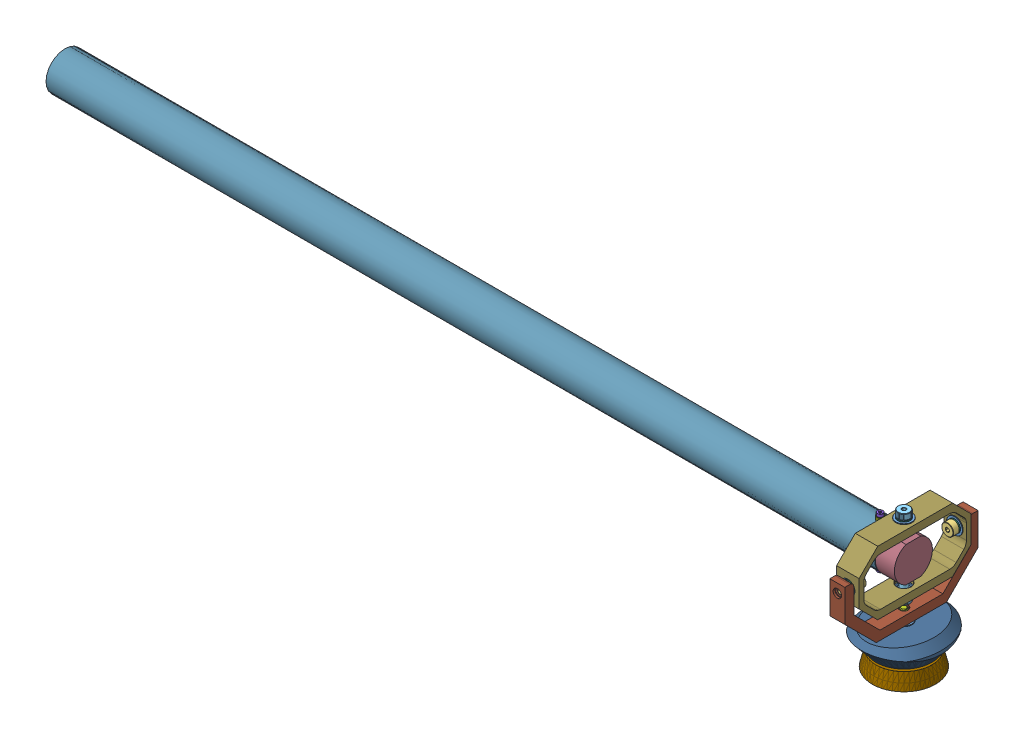
SolidWorks assembly WandMountB, configuration Default. Lengths in mm.
Overall size (585.53 95.36 89).
41 component instances, 17 part files, 91 mates.
Components (placement in the parent):
- 57155K301_Stainless Steel Ball BearingB-1: 57155K301_Stainless Steel Ball BearingB [57155K301] at (0 73.0039 0) x (-0.175436 0 0.984491) z (0 -1 0) size (10.72 10.72 3.17)
- 57155K301_Stainless Steel Ball BearingB-2: 57155K301_Stainless Steel Ball BearingB [57155K301] at (0 32.5996 0) x (-0.999998 0 0.001816) z (0 1 0) size (10.72 10.72 3.17)
- 57155K301_Stainless Steel Ball BearingB-3: 57155K301_Stainless Steel Ball BearingB [57155K301] at (0 52.8017 -35.371) x (-0.957901 0.287097 0) z (0 0 -1) size (10.72 10.72 3.17)
- 57155K301_Stainless Steel Ball BearingB-4: 57155K301_Stainless Steel Ball BearingB [57155K301] at (0 52.8017 35.371) x (-0.999998 -0.001816 0) z (0 0 1) size (10.72 10.72 3.17)
- 94459A310_Heat-Set Inserts for PlasticB-3: 94459A310_Heat-Set Inserts for PlasticB [94459A310] at (0 52.8017 43.199) x (0.931607 0.363468 0) z (-0.363468 0.931607 0) size (6.45 5.21 6.45)
- 94459A310_Heat-Set Inserts for PlasticB-4: 94459A310_Heat-Set Inserts for PlasticB [94459A310] at (0 52.8017 -43.199) x (0.553148 0.833083 0) z (0.833083 -0.553148 0) size (6.45 5.21 6.45)
- 94459A310_Heat-Set Inserts for PlasticB-5: 94459A310_Heat-Set Inserts for PlasticB [94459A310] at (0 21.0008 0) x (-0.969537 0 -0.244946) z (-0.244946 0 0.969537) size (6.45 5.21 6.45)
- 57155K301_Stainless Steel Ball BearingB-5: 57155K301_Stainless Steel Ball BearingB [57155K301] at (0 1.0795 0) x (-0.199974 0 0.979801) z (0 1 0) size (10.72 10.72 3.17)
- 57155K301_Stainless Steel Ball BearingB-6: 57155K301_Stainless Steel Ball BearingB [57155K301] at (0 13.9205 0) x (0.455162 0 -0.890409) z (0 -1 0) size (10.72 10.72 3.17)
- 93985A202_High-Strength 416 Stainless Steel Precision Shoulder ScrewB-1: 93985A202_High-Strength 416 Stainless Steel Precision Shoulder ScrewB [93985A202] at (0 52.8017 29.021) x (0.127636 -0.991821 0) z (0 0 -1) size (7.94 7.94 13.94)
- 93985A202_High-Strength 416 Stainless Steel Precision Shoulder ScrewB-2: 93985A202_High-Strength 416 Stainless Steel Precision Shoulder ScrewB [93985A202] at (0 52.8017 -29.021) x (-1 0 0) z (0 0 1) size (7.94 7.94 13.94)
- 94459A310_Heat-Set Inserts for PlasticB-1: 94459A310_Heat-Set Inserts for PlasticB [94459A310] at (0 4.699 -12.5) x (0.43803 0 0.898961) z (0.898961 0 -0.43803) size (6.45 5.21 6.45)
- 94459A310_Heat-Set Inserts for PlasticB-2: 94459A310_Heat-Set Inserts for PlasticB [94459A310] at (0 4.699 12.5) x (0.130741 0 -0.991417) z (-0.991417 0 -0.130741) size (6.45 5.21 6.45)
- 94459A310_Heat-Set Inserts for PlasticB-7: 94459A310_Heat-Set Inserts for PlasticB [94459A310] at (0 45.8008 0) x (-0.378851 0 0.925458) z (0.925458 0 0.378851) size (6.45 5.21 6.45)
- 94459A310_Heat-Set Inserts for PlasticB-9: 94459A310_Heat-Set Inserts for PlasticB [94459A310] at (0 59.8028 0) x (0.992335 0 0.123574) z (-0.123574 0 0.992335) size (6.45 5.21 6.45)
- 91251A196_Black-Oxide Alloy Steel Socket Head Screw-1: 91251A196_Black-Oxide Alloy Steel Socket Head Screw [91251A196] at (0 -5.6453 12.5) x (0.587183 0 -0.809454) z (0 -1 0) size (6.86 6.86 20.6)
- 91251A196_Black-Oxide Alloy Steel Socket Head Screw-2: 91251A196_Black-Oxide Alloy Steel Socket Head Screw [91251A196] at (0 -5.6453 -12.5) x (0.424116 0 -0.905608) z (0 -1 0) size (6.86 6.86 20.6)
- 91259A507_Alloy Steel Shoulder Screw-1: 91259A507_Alloy Steel Shoulder Screw [91259A507] at (0 26.2496 0) x (0.715485 0 -0.698628) z (0 -1 0) size (7.94 7.94 18.7)
- 91259A507_Alloy Steel Shoulder Screw-2: 91259A507_Alloy Steel Shoulder Screw [91259A507] at (0 79.3539 0) x (0.999986 0 -0.005203) z (0 1 0) size (7.94 7.94 18.7)
- 94459A418_Heat-Set Inserts for PlasticP3B-5: 94459A418_Heat-Set Inserts for PlasticP3B [94459A418] at (-15.875 58.8143 0) x (-0.328275 0 -0.944582) z (0.944582 0 -0.328275) size (3.8 4.42 3.8)
- 94459A418_Heat-Set Inserts for PlasticP3B-6: 94459A418_Heat-Set Inserts for PlasticP3B [94459A418] at (-15.875 46.7892 0) x (0.706646 0 -0.707568) z (-0.707568 0 -0.706646) size (3.8 4.42 3.8)
- 93985A207_High-Strength 416 Stainless Steel Precision Shoulder ScrewB-1: 93985A207_High-Strength 416 Stainless Steel Precision Shoulder ScrewB [93985A207] at (0 -5.2705 0) x (-0.546944 0 -0.837169) z (0 -1 0) size (7.94 7.94 28.23)
- 91290A015_Black-Oxide Alloy Steel Socket Head Screw-1: 91290A015_Black-Oxide Alloy Steel Socket Head Screw [91290A015] at (-15.875 40.8027 0) x (-0.748479 0 0.663158) z (0 -1 0) size (3.8 3.8 10.09)
- 91290A015_Black-Oxide Alloy Steel Socket Head Screw-2: 91290A015_Black-Oxide Alloy Steel Socket Head Screw [91290A015] at (-15.875 64.8008 0) x (-0.850889 0 0.525346) z (0 1 0) size (3.8 3.8 10.09)
- Vive Controller 1.5B-1: Vive Controller 1.5B [Default] at (0.0016 6.0546 36.5874) x (1 -0.000227 0) z (-0.000192 -0.847056 0.531504) size (118.44 84.37 219.45) (hidden)
- BottomPlugB-2: BottomPlugB [Default] at origin size (42.24 11.38 42.24)
- TopPlugB-2: TopPlugB [Default] at origin size (50.17 16.12 56.99)
- GimbalArcP3B-1: GimbalArcP3B [Default] at (5 52.8017 0) x (0 0 -1) z (-1 0 0) size (89 42.5 10)
- GimbalRingP3B-1: GimbalRingP3B [Default] at (7.5 52.8017 0) x (0 0 -1) z (0 1 0) size (74.93 15 42.56)
- GimbalPlugP3B-2: GimbalPlugP3B [Default] at (6.35 52.8017 0) x (0 -1 0) z (0 0 -1) size (23.4 25.4 25.4)
- MainTubeP3-1: MainTubeP3 [Default] at (-6.875 52.8017 0) x (0 -1 0) z (-1 0 0) size (25.4 25.4 553.63)
- GimbalSpacerP3B-1: GimbalSpacerP3B [Default] at (0 52.8017 -32.9897) x (0 0 -1) z (-0.964268 0.264928 0) size (0.79 8 8)
- GimbalSpacerP3B-2: GimbalSpacerP3B [Default] at (0 52.8017 -36.9585) x (0 0 -1) z (-0.964268 0.264928 0) size (0.79 8 8)
- GimbalSpacerP3B-3: GimbalSpacerP3B [Default] at (0 52.8017 32.9897) x (0 0 1) z (0.64176 0.766906 0) size (0.79 8 8)
- GimbalSpacerP3B-4: GimbalSpacerP3B [Default] at (0 52.8017 36.9585) x (0 0 1) z (0.64176 0.766906 0) size (0.79 8 8)
- GimbalSpacerP3B-5: GimbalSpacerP3B [Default] at (0 16.3018 0) x (0 -1 0) z (0.658931 0 0.752203) size (0.79 8 8)
- GimbalSpacerP3B-6: GimbalSpacerP3B [Default] at (0 -0.508 0) x (0 -1 0) z (0.795265 0 0.606261) size (0.79 8 8)
- GimbalSpacerP3B-7: GimbalSpacerP3B [Default] at (0 75.3851 0) x (0 -1 0) z (0.998677 0 -0.051423) size (0.79 8 8)
- GimbalSpacerP3B-8: GimbalSpacerP3B [Default] at (0 31.0121 0) x (0 -1 0) z (0.998677 0 -0.051423) size (0.79 8 8)
- ClampSpacer-1: ClampSpacer [Default] at (-15.875 65.3008 0) x (0 1 0) z (0 0 1) size (2.63 4.5 4.5)
- ClampSpacer-2: ClampSpacer [Default] at (-15.875 40.3027 0) x (0 -1 0) z (0 0 -1) size (2.63 4.5 4.5)
Mates (geometry in assembly coordinates):
- Coincident5: coincident aligned: plane of Vive Controller 1.5-1 through (0.0016 0 36.5874) normal (0 1 0)
- Coincident4: coordinate: point of BottomPlug-2
- Coincident6: coincident: line of Vive Controller 1.5-1 through (0 0 0) axis (0 1 0)
- Coincident7: coincident: line of Vive Controller 1.5-1 through (0 0 0) axis (0 1 0)
- Parallel1: parallel anti-aligned: plane of Vive Controller 1.5-1 through (0.0016 6.0546 -0.0032) normal (0 0 -1)
- Coincident9: coordinate: unknown of TopPlugB-2
- Concentric3: concentric anti-aligned: cylinder of BottomPlugB-2 through (0 -11.5 -12.5) axis (0 -1 0) radius 2.2479; cylinder of 94459A310_Heat-Set Inserts for PlasticB-1 through (0 4.699 -12.5) axis (0 1 0) radius 2.7686
- Concentric4: concentric anti-aligned: cylinder of BottomPlugB-2 through (0 -11.5 12.5) axis (0 -1 0) radius 2.2479; cylinder of 94459A310_Heat-Set Inserts for PlasticB-2 through (0 4.699 12.5) axis (0 1 0) radius 2.7686
- Concentric2: concentric anti-aligned: cylinder of GimbalRingP3B-1 through (0 31.5191 0) axis (0 1 0) radius 4.7625; cylinder of 57155K301_Stainless Steel Ball BearingB-1 through (0 73.0039 0) axis (0 -1 0) radius 4.7625
- Coincident1: coincident anti-aligned: plane of GimbalRingP3B-1 through (-7.5 74.0834 0) normal (0 1 0); plane of 57155K301_Stainless Steel Ball BearingB-1 through (-5.2763 74.0834 -0.9402) normal (0 -1 0)
- Coincident26: coincident anti-aligned: plane of 57155K301_Stainless Steel Ball BearingB-1 through (-3.0476 74.5914 -0.5431) normal (0 1 0); plane of GimbalSpacerP3B-7 through (0 74.5914 0) normal (0 -1 0)
- Concentric34: concentric anti-aligned: cylinder of GimbalRingP3B-1 through (0 74.0844 0) axis (0 -1 0) radius 4.7625; cylinder of 57155K301_Stainless Steel Ball BearingB-2 through (0 32.5996 0) axis (0 1 0) radius 4.7625
- Coincident2: coincident anti-aligned: plane of GimbalRingP3B-1 through (-7.5 31.5201 0) normal (0 -1 0); plane of 57155K301_Stainless Steel Ball BearingB-2 through (0.0097 31.5201 5.3594) normal (0 1 0)
- Coincident27: coincident anti-aligned: plane of 57155K301_Stainless Steel Ball BearingB-2 through (0.0056 31.0121 3.0956) normal (0 -1 0); plane of GimbalSpacerP3B-8 through (0 31.0121 0) normal (0 1 0)
- Concentric6: concentric anti-aligned: cylinder of GimbalRingP3B-1 through (0 52.8017 -37.4675) axis (0 0 1) radius 4.7625; cylinder of 57155K301_Stainless Steel Ball BearingB-3 through (0 52.8017 -35.371) axis (0 0 -1) radius 4.7625
- Coincident28: coincident anti-aligned: plane of GimbalRingP3B-1 through (-7.5 52.8017 -34.2915) normal (0 0 1); plane of 57155K301_Stainless Steel Ball BearingB-3 through (1.5387 57.9355 -34.2915) normal (0 0 -1)
- Coincident29: coincident anti-aligned: plane of 57155K301_Stainless Steel Ball BearingB-3 through (0.8887 55.7671 -33.7835) normal (0 0 1); plane of GimbalSpacerP3B-1 through (0 52.8017 -33.7835) normal (0 0 -1)
- Coincident10: coincident anti-aligned: plane of 57155K301_Stainless Steel Ball BearingB-3 through (0.6837 55.0828 -36.9585) normal (0 0 -1); plane of GimbalSpacerP3B-2 through (0 52.8017 -36.9585) normal (0 0 1)
- Concentric41: concentric aligned: cylinder of 57155K301_Stainless Steel Ball BearingB-3 through (0 52.8017 -35.371) axis (0 0 -1) radius 2.3813; cylinder of 93985A202_High-Strength 416 Stainless Steel Precision Shoulder ScrewB-2 through (0 52.8017 -42.5147) axis (0 0 -1) radius 2.3813
- Concentric7: concentric anti-aligned: cylinder of GimbalRingP3B-1 through (0 52.8017 37.4675) axis (0 0 -1) radius 4.7625; cylinder of 57155K301_Stainless Steel Ball BearingB-4 through (0 52.8017 35.371) axis (0 0 1) radius 4.7625
- Coincident30: coincident anti-aligned: plane of GimbalRingP3B-1 through (-7.5 52.8017 34.2915) normal (0 0 -1); plane of 57155K301_Stainless Steel Ball BearingB-4 through (0.0097 47.4424 34.2915) normal (0 0 1)
- Coincident31: coincident anti-aligned: plane of 57155K301_Stainless Steel Ball BearingB-4 through (0.0056 49.7061 33.7835) normal (0 0 -1); plane of GimbalSpacerP3B-3 through (0 52.8017 33.7835) normal (0 0 1)
- Coincident13: coincident anti-aligned: plane of 57155K301_Stainless Steel Ball BearingB-4 through (0.0043 50.4205 36.9585) normal (0 0 1); plane of GimbalSpacerP3B-4 through (0 52.8017 36.9585) normal (0 0 -1)
- Concentric37: concentric aligned: cylinder of 57155K301_Stainless Steel Ball BearingB-4 through (0 52.8017 35.371) axis (0 0 1) radius 2.3813; cylinder of 93985A202_High-Strength 416 Stainless Steel Precision Shoulder ScrewB-1 through (0 52.8017 42.5147) axis (0 0 1) radius 2.3813
- Coincident14: coincident aligned: plane of GimbalArcP3B-1 through (-5 58.8017 38.5) normal (0 0 -1); plane of 94459A310_Heat-Set Inserts for PlasticB-3 through (2.946 53.9511 38.5) normal (0 0 -1)
- Concentric16: concentric anti-aligned: cylinder of 94459A310_Heat-Set Inserts for PlasticB-3 through (0 52.8017 43.199) axis (0 0 1) radius 2.7686; cylinder of GimbalArcP3B-1 through (0 52.8017 44.5) axis (0 0 -1) radius 2.8067
- Concentric40: concentric aligned: cylinder of 94459A310_Heat-Set Inserts for PlasticB-3 through (0 52.8017 43.199) axis (0 0 1) radius 2.7686; cylinder of 93985A202_High-Strength 416 Stainless Steel Precision Shoulder ScrewB-1 through (0 52.8017 42.5147) axis (0 0 1) radius 2.3813
- Coincident15: coincident aligned: plane of GimbalArcP3B-1 through (-5 39.8017 -38.5) normal (0 0 1); plane of 94459A310_Heat-Set Inserts for PlasticB-4 through (1.7492 55.4362 -38.5) normal (0 0 1)
- Concentric17: concentric anti-aligned: cylinder of GimbalArcP3B-1 through (0 52.8017 -44.5) axis (0 0 1) radius 2.8067; cylinder of 94459A310_Heat-Set Inserts for PlasticB-4 through (0 52.8017 -43.199) axis (0 0 -1) radius 2.7686
- Concentric43: concentric aligned: cylinder of 94459A310_Heat-Set Inserts for PlasticB-4 through (0 52.8017 -43.199) axis (0 0 -1) radius 2.7686; cylinder of 93985A202_High-Strength 416 Stainless Steel Precision Shoulder ScrewB-2 through (0 52.8017 -42.5147) axis (0 0 -1) radius 2.3813
- Coincident16: coincident aligned: plane of GimbalArcP3B-1 through (-5 16.3018 -23.4853) normal (0 -1 0); plane of 94459A310_Heat-Set Inserts for PlasticB-5 through (-3.066 16.3018 -0.7746) normal (0 -1 0)
- Concentric18: concentric aligned: cylinder of GimbalArcP3B-1 through (0 16.3018 0) axis (0 1 0) radius 2.8067; cylinder of 94459A310_Heat-Set Inserts for PlasticB-5 through (0 21.0008 0) axis (0 1 0) radius 2.7686
- Coincident19: coincident anti-aligned: plane of 94459A310_Heat-Set Inserts for PlasticB-5 through (-3.066 16.3018 -0.7746) normal (0 -1 0); plane of GimbalSpacerP3B-5 through (0 16.3018 0) normal (0 1 0)
- Concentric49: concentric aligned: cylinder of 94459A310_Heat-Set Inserts for PlasticB-5 through (0 21.0008 0) axis (0 1 0) radius 2.7686; cylinder of 93985A207_High-Strength 416 Stainless Steel Precision Shoulder ScrewB-1 through (0 22.5107 0) axis (0 1 0) radius 2.3813
- Concentric24: concentric aligned: cylinder of 57155K301_Stainless Steel Ball BearingB-5 through (0 1.0795 0) axis (0 1 0) radius 2.3813; cylinder of GimbalSpacerP3B-6 through (0 -1.3017 0) axis (0 1 0) radius 2.3813
- Coincident22: coincident anti-aligned: plane of 57155K301_Stainless Steel Ball BearingB-5 through (3.0331 -0.508 0.619) normal (0 -1 0); plane of GimbalSpacerP3B-6 through (0 -0.508 0) normal (0 1 0)
- Concentric45: concentric aligned: cylinder of 57155K301_Stainless Steel Ball BearingB-5 through (0 1.0795 0) axis (0 1 0) radius 2.3813; cylinder of 93985A207_High-Strength 416 Stainless Steel Precision Shoulder ScrewB-1 through (0 22.5107 0) axis (0 1 0) radius 2.3813
- Concentric23: concentric anti-aligned: cylinder of 57155K301_Stainless Steel Ball BearingB-6 through (0 13.9205 0) axis (0 -1 0) radius 2.3813; cylinder of GimbalSpacerP3B-5 through (0 15.508 0) axis (0 1 0) radius 2.3813
- Coincident20: coincident anti-aligned: plane of 57155K301_Stainless Steel Ball BearingB-6 through (2.7564 15.508 1.409) normal (0 1 0); plane of GimbalSpacerP3B-5 through (0 15.508 0) normal (0 -1 0)
- Concentric47: concentric anti-aligned: cylinder of 57155K301_Stainless Steel Ball BearingB-6 through (0 13.9205 0) axis (0 -1 0) radius 2.3813; cylinder of 93985A207_High-Strength 416 Stainless Steel Precision Shoulder ScrewB-1 through (0 22.5107 0) axis (0 1 0) radius 2.3813
- Concentric38: concentric anti-aligned: cylinder of GimbalSpacerP3B-3 through (0 52.8017 33.7835) axis (0 0 -1) radius 2.3813; cylinder of 93985A202_High-Strength 416 Stainless Steel Precision Shoulder ScrewB-1 through (0 52.8017 42.5147) axis (0 0 1) radius 2.3813
- Concentric39: concentric anti-aligned: cylinder of GimbalSpacerP3B-4 through (0 52.8017 37.7522) axis (0 0 -1) radius 2.3813; cylinder of 93985A202_High-Strength 416 Stainless Steel Precision Shoulder ScrewB-1 through (0 52.8017 42.5147) axis (0 0 1) radius 2.3813
- Coincident36: coincident anti-aligned: plane of GimbalSpacerP3B-3 through (0 52.8017 32.9897) normal (0 0 -1); plane of 93985A202_High-Strength 416 Stainless Steel Precision Shoulder ScrewB-1 through (3.9363 53.3083 32.9897) normal (0 0 1)
- Concentric42: concentric anti-aligned: cylinder of GimbalSpacerP3B-1 through (0 52.8017 -33.7835) axis (0 0 1) radius 2.3813; cylinder of 93985A202_High-Strength 416 Stainless Steel Precision Shoulder ScrewB-2 through (0 52.8017 -42.5147) axis (0 0 -1) radius 2.3813
- Coincident37: coincident anti-aligned: plane of GimbalSpacerP3B-1 through (0 52.8017 -32.9897) normal (0 0 1); plane of 93985A202_High-Strength 416 Stainless Steel Precision Shoulder ScrewB-2 through (0 56.7705 -32.9897) normal (0 0 -1)
- Concentric44: concentric anti-aligned: cylinder of GimbalSpacerP3B-2 through (0 52.8017 -37.7522) axis (0 0 1) radius 2.3813; cylinder of 93985A202_High-Strength 416 Stainless Steel Precision Shoulder ScrewB-2 through (0 52.8017 -42.5147) axis (0 0 -1) radius 2.3813
- Width1: width anti-aligned: plane of GimbalArcP3B-1 through (-5 58.8017 38.5) normal (0 0 -1); plane of GimbalRingP3B-1 through (-5 39.8017 -38.5) normal (0 0 1); plane of GimbalArcP3B-1 through (-7.5 52.8017 37.4665) normal (0 0 1); plane of GimbalRingP3B-1 through (-7.5 52.8017 -37.4665) normal (0 0 -1)
- Concentric22: concentric aligned: cylinder of GimbalArcP3B-1 through (0 16.3018 0) axis (0 1 0) radius 2.8067; cylinder of GimbalSpacerP3B-5 through (0 15.508 0) axis (0 1 0) radius 2.3813
- Concentric48: concentric aligned: cylinder of GimbalSpacerP3B-5 through (0 15.508 0) axis (0 1 0) radius 2.3813; cylinder of 93985A207_High-Strength 416 Stainless Steel Precision Shoulder ScrewB-1 through (0 22.5107 0) axis (0 1 0) radius 2.3813
- Concentric46: concentric aligned: cylinder of GimbalSpacerP3B-6 through (0 -1.3017 0) axis (0 1 0) radius 2.3813; cylinder of 93985A207_High-Strength 416 Stainless Steel Precision Shoulder ScrewB-1 through (0 22.5107 0) axis (0 1 0) radius 2.3813
- Coincident38: coincident anti-aligned: plane of GimbalSpacerP3B-6 through (0 -1.3017 0) normal (0 -1 0); plane of 93985A207_High-Strength 416 Stainless Steel Precision Shoulder ScrewB-1 through (-3.3225 -1.3017 2.1707) normal (0 1 0)
- Angle2: planar angle = 0.872665 rad: plane of assembly through (0 0 0) normal (0 1 0); plane of assembly; plane of GimbalRingP3B-1 through (7.5 52.8017 0) normal (-1 0 0)
- Coincident39: coincident aligned: plane of TopPlugB-2 through (0 0 0) normal (0 -1 0); plane of 94459A310_Heat-Set Inserts for PlasticB-2 through (0.4134 0 9.3648) normal (0 -1 0)
- Concentric54: concentric anti-aligned: cylinder of TopPlugB-2 through (0 5.5 -12.5) axis (0 -1 0) radius 2.8067; cylinder of 94459A310_Heat-Set Inserts for PlasticB-1 through (0 4.699 -12.5) axis (0 1 0) radius 2.7686
- Coincident40: coincident aligned: plane of TopPlugB-2 through (0 0 0) normal (0 -1 0); plane of 94459A310_Heat-Set Inserts for PlasticB-1 through (1.3852 0 -9.6572) normal (0 -1 0)
- Concentric55: concentric anti-aligned: cylinder of TopPlugB-2 through (0 5.5 12.5) axis (0 -1 0) radius 2.8067; cylinder of 94459A310_Heat-Set Inserts for PlasticB-2 through (0 4.699 12.5) axis (0 1 0) radius 2.7686
- Concentric56: concentric anti-aligned: cylinder of TopPlugB-2 through (0 3.5 0) axis (0 -1 0) radius 4.7625; cylinder of 57155K301_Stainless Steel Ball BearingB-5 through (0 1.0795 0) axis (0 1 0) radius 4.7625
- Coincident41: coincident anti-aligned: plane of TopPlugB-2 through (0 0 0) normal (0 -1 0); plane of 57155K301_Stainless Steel Ball BearingB-5 through (5.2511 0 1.0717) normal (0 1 0)
- Concentric57: concentric anti-aligned: cylinder of TopPlugB-2 through (0 11.5 0) axis (0 1 0) radius 4.7625; cylinder of 57155K301_Stainless Steel Ball BearingB-6 through (0 13.9205 0) axis (0 -1 0) radius 4.7625
- Coincident42: coincident anti-aligned: plane of TopPlugB-2 through (0 15 0) normal (0 1 0); plane of 57155K301_Stainless Steel Ball BearingB-6 through (4.7721 15 2.4394) normal (0 -1 0)
- Concentric58: concentric anti-aligned: cylinder of 57155K301_Stainless Steel Ball BearingB-1 through (0 73.0039 0) axis (0 -1 0) radius 2.3813; cylinder of GimbalPlugP3B-2 through (0 40.1017 0) axis (0 1 0) radius 2.8067
- Symmetric1: symmetric aligned: plane of GimbalRingP3B-1 through (-7.5 36.6951 0) normal (0 1 0); plane of GimbalPlugP3B-2 through (-7.5 68.9084 0) normal (0 -1 0); plane of GimbalRingP3B-1 through (6.35 52.8017 0) normal (0 -1 0)
- Concentric59: concentric aligned: cylinder of GimbalPlugP3B-2 through (0 40.1017 0) axis (0 1 0) radius 2.8067; cylinder of 94459A310_Heat-Set Inserts for PlasticB-7 through (0 45.8008 0) axis (0 1 0) radius 2.7686
- Coincident48: coincident aligned: plane of GimbalPlugP3B-2 through (-19.05 41.1018 0) normal (0 -1 0); plane of 94459A310_Heat-Set Inserts for PlasticB-7 through (-1.198 41.1018 2.9266) normal (0 -1 0)
- Concentric60: concentric anti-aligned: cylinder of GimbalPlugP3B-2 through (0 40.1017 0) axis (0 1 0) radius 2.8067; cylinder of 94459A310_Heat-Set Inserts for PlasticB-9 through (0 59.8028 0) axis (0 -1 0) radius 2.7686
- Coincident47: coincident aligned: plane of GimbalPlugP3B-2 through (-19.05 64.5018 0) normal (0 1 0); plane of 94459A310_Heat-Set Inserts for PlasticB-9 through (3.1381 64.5018 0.3908) normal (0 1 0)
- Concentric61: concentric anti-aligned: cylinder of 57155K301_Stainless Steel Ball BearingB-1 through (0 73.0039 0) axis (0 -1 0) radius 2.3813; cylinder of GimbalSpacerP3B-7 through (0 74.5914 0) axis (0 1 0) radius 2.3813
- Concentric62: concentric aligned: cylinder of 57155K301_Stainless Steel Ball BearingB-2 through (0 32.5996 0) axis (0 1 0) radius 2.3813; cylinder of GimbalSpacerP3B-8 through (0 30.2184 0) axis (0 1 0) radius 2.3813
- Concentric63: concentric anti-aligned: cylinder of BottomPlugB-2 through (0 -11.5 12.5) axis (0 -1 0) radius 2.2479; cylinder of 91251A196_Black-Oxide Alloy Steel Socket Head Screw-1 through (0 4.375 12.5) axis (0 1 0) radius 3.429
- Coincident43: coincident anti-aligned: plane of BottomPlugB-2 through (0 -11.5 0) normal (0 -1 0); plane of 91251A196_Black-Oxide Alloy Steel Socket Head Screw-1 through (2.4384 -11.5 14.2689) normal (0 1 0)
- Concentric64: concentric anti-aligned: cylinder of BottomPlugB-2 through (0 -11.5 -12.5) axis (0 -1 0) radius 2.2479; cylinder of 91251A196_Black-Oxide Alloy Steel Socket Head Screw-2 through (0 4.375 -12.5) axis (0 1 0) radius 3.429
- Coincident44: coincident anti-aligned: plane of BottomPlugB-2 through (0 -11.5 0) normal (0 -1 0); plane of 91251A196_Black-Oxide Alloy Steel Socket Head Screw-2 through (2.7281 -11.5 -11.2224) normal (0 1 0)
- Concentric65: concentric aligned: cylinder of 57155K301_Stainless Steel Ball BearingB-2 through (0 32.5996 0) axis (0 1 0) radius 2.3813; cylinder of 91259A507_Alloy Steel Shoulder Screw-1 through (0 44.5059 0) axis (0 1 0) radius 2.3813
- Coincident45: coincident anti-aligned: plane of GimbalSpacerP3B-8 through (0 30.2184 0) normal (0 -1 0); plane of 91259A507_Alloy Steel Shoulder Screw-1 through (-2.7727 30.2184 -2.8396) normal (0 1 0)
- Concentric66: concentric aligned: cylinder of 57155K301_Stainless Steel Ball BearingB-1 through (0 73.0039 0) axis (0 -1 0) radius 2.3813; cylinder of 91259A507_Alloy Steel Shoulder Screw-2 through (0 61.0976 0) axis (0 -1 0) radius 2.3813
- Coincident46: coincident anti-aligned: plane of GimbalSpacerP3B-7 through (0 75.3851 0) normal (0 1 0); plane of 91259A507_Alloy Steel Shoulder Screw-2 through (0.0207 75.3851 3.9687) normal (0 -1 0)
- Coincident49: coincident aligned: plane of GimbalPlugP3B-2 through (-19.05 62.9143 0) normal (0 1 0); plane of 94459A418_Heat-Set Inserts for PlasticP3B-5 through (-16.4872 62.9143 -1.7616) normal (0 1 0)
- Coincident50: coincident aligned: plane of GimbalPlugP3B-2 through (-19.05 42.6893 0) normal (0 -1 0); plane of 94459A418_Heat-Set Inserts for PlasticP3B-6 through (-14.5571 42.6893 -1.3196) normal (0 -1 0)
- Concentric69: concentric aligned: line of GimbalPlugP3B-2 through (-15.875 52.8017 0) axis (0 -1 0); cylinder of 94459A418_Heat-Set Inserts for PlasticP3B-5 through (-15.875 58.8143 0) axis (0 -1 0) radius 1.535
- Concentric70: concentric anti-aligned: line of GimbalPlugP3B-2 through (-15.875 52.8017 0) axis (0 -1 0); cylinder of 94459A418_Heat-Set Inserts for PlasticP3B-6 through (-15.875 46.7892 0) axis (0 1 0) radius 1.535
- Concentric71: concentric aligned: cylinder of GimbalPlugP3B-2 through (1006.35 52.8017 0) axis (1 0 0) radius 11.1125; cylinder of MainTubeP3-1 through (-560.505 52.8017 0) axis (1 0 0) radius 11.6205
- Concentric73: concentric anti-aligned: line of GimbalPlugP3B-2 through (-15.875 52.8017 0) axis (0 -1 0); cylinder of MainTubeP3-1 through (-15.875 52.8017 0) axis (0 1 0) radius 1.2
- Concentric74: concentric anti-aligned: cylinder of ClampSpacer-1 through (2.5717 63.7565 -7.2298) axis (0.19228 0.81905 -0.540542) radius 12.7; cylinder of MainTubeP3-1 through (107.7738 511.8832 -302.9767) axis (-0.19228 -0.81905 0.540542) radius 12.7
- Concentric75: concentric aligned: line of GimbalPlugP3B-2 through (-15.875 52.8017 0) axis (0 -1 0); cylinder of ClampSpacer-1 through (-15.875 67.8008 0) axis (0 -1 0) radius 1.1
- Concentric76: concentric anti-aligned: cylinder of ClampSpacer-1 through (-13.625 52.8017 0) axis (-1 0 0) radius 12.7; cylinder of MainTubeP3-1 through (-560.505 52.8017 0) axis (1 0 0) radius 12.7
- Concentric77: concentric anti-aligned: line of GimbalPlugP3B-2 through (-15.875 52.8017 0) axis (0 -1 0); cylinder of ClampSpacer-2 through (-15.875 37.8027 0) axis (0 1 0) radius 1.1
- Concentric79: concentric anti-aligned: cylinder of MainTubeP3-1 through (-560.505 52.8017 0) axis (1 0 0) radius 12.7; cylinder of ClampSpacer-2 through (-13.625 52.8017 0) axis (-1 0 0) radius 12.7
- Concentric80: concentric anti-aligned: line of GimbalPlugP3B-2 through (-15.875 52.8017 0) axis (0 -1 0); cylinder of 91290A015_Black-Oxide Alloy Steel Socket Head Screw-1 through (-15.875 45.8027 0) axis (0 1 0) radius 1.9
- Coincident52: coincident anti-aligned: plane of ClampSpacer-2 through (-15.875 37.8027 0) normal (0 -1 0); plane of 91290A015_Black-Oxide Alloy Steel Socket Head Screw-1 through (-17.0687 37.8027 -1.3473) normal (0 1 0)
- Concentric81: concentric aligned: line of GimbalPlugP3B-2 through (-15.875 52.8017 0) axis (0 -1 0); cylinder of 91290A015_Black-Oxide Alloy Steel Socket Head Screw-2 through (-15.875 59.8008 0) axis (0 -1 0) radius 1.9
- Coincident53: coincident anti-aligned: plane of ClampSpacer-1 through (-15.875 67.8008 0) normal (0 1 0); plane of 91290A015_Black-Oxide Alloy Steel Socket Head Screw-2 through (-14.9294 67.8008 1.5316) normal (0 -1 0)
